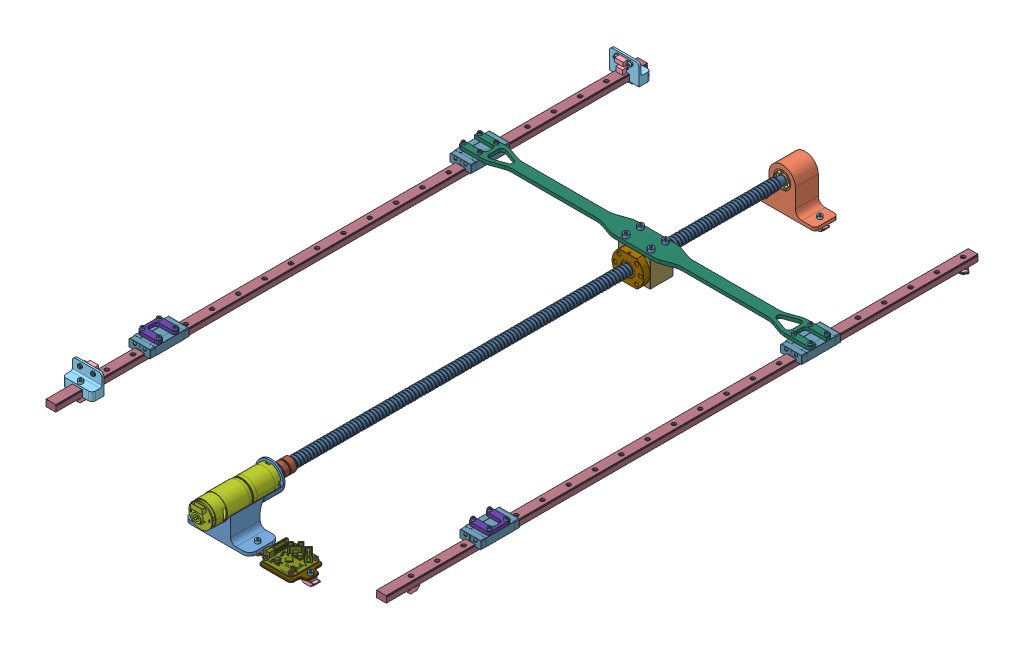
SolidWorks assembly Montaje_Eje_Z_Unity, configuration Predeterminado. Lengths in mm.
Overall size (541.5 84.7 933.8).
85 component instances, 23 part files, 191 mates.
Components (placement in the parent):
- socket head cap screw_iso2-2: socket head cap screw_iso2 [ISO 4762 M3 x 8 - 8N] at (-240.4498 15.8322 -56.4995) x (0 -1 0) z (0 0 1) size (11 5.5 5.5)
- socket head cap screw_iso2-3: socket head cap screw_iso2 [ISO 4762 M3 x 8 - 8N] at (-215.4498 15.8322 -31.4995) x (0 -1 0) z (0 0 1) size (11 5.5 5.5)
- socket head cap screw_iso2-4: socket head cap screw_iso2 [ISO 4762 M3 x 8 - 8N] at (-240.4498 15.8322 -31.4995) x (0 -1 0) z (0 0 1) size (11 5.5 5.5)
- socket head cap screw_iso2-5: socket head cap screw_iso2 [ISO 4762 M3 x 8 - 8N] at (-215.4498 15.8322 -56.4995) x (0 -1 0) z (0.194661 0 0.98087) size (11 5.5 5.5)
- socket head cap screw_iso2-6: socket head cap screw_iso2 [ISO 4762 M3 x 8 - 8N] at (287.5502 15.8322 -56.4995) x (0 -1 0) z (0.194661 0 0.98087) size (11 5.5 5.5)
- socket head cap screw_iso2-7: socket head cap screw_iso2 [ISO 4762 M3 x 8 - 8N] at (262.5502 15.8322 -31.4995) x (0 -1 0) z (0 0 1) size (11 5.5 5.5)
- socket head cap screw_iso2-8: socket head cap screw_iso2 [ISO 4762 M3 x 8 - 8N] at (287.5502 15.8322 -31.4995) x (0 -1 0) z (-0.140271 0 0.990113) size (11 5.5 5.5)
- socket head cap screw_iso2-9: socket head cap screw_iso2 [ISO 4762 M3 x 8 - 8N] at (262.5502 15.8322 -56.4995) x (0 -1 0) z (-0.070011 0 0.997546) size (11 5.5 5.5)
- socket head cap screw_iso2-10: socket head cap screw_iso2 [ISO 4762 M5 x 16 - 16N] at (43.5502 17.8322 -54.9995) x (0 -1 0) z (0 0 1) size (21 8.5 8.5)
- socket head cap screw_iso2-11: socket head cap screw_iso2 [ISO 4762 M5 x 16 - 16N] at (43.5502 17.8322 -32.9995) x (0 -1 0) z (0.965322 0 -0.261062) size (21 8.5 8.5)
- socket head cap screw_iso2-12: socket head cap screw_iso2 [ISO 4762 M5 x 16 - 16N] at (5.5502 17.8322 -32.9995) x (0 -1 0) z (0 0 1) size (21 8.5 8.5)
- socket head cap screw_iso2-13: socket head cap screw_iso2 [ISO 4762 M5 x 16 - 16N] at (5.5502 17.8322 -54.9995) x (0 -1 0) z (0 0 1) size (21 8.5 8.5)
- socket head cap screw_iso2-23: socket head cap screw_iso2 [ISO 4762 M3 x 8 - 8N] at (287.5502 15.8322 456.5005) x (0 -1 0) z (0 0 1) size (11 5.5 5.5)
- socket head cap screw_iso2-24: socket head cap screw_iso2 [ISO 4762 M3 x 8 - 8N] at (287.5502 15.8322 431.5005) x (0 -1 0) z (0 0 1) size (11 5.5 5.5)
- socket head cap screw_iso2-25: socket head cap screw_iso2 [ISO 4762 M3 x 8 - 8N] at (262.5502 15.8322 456.5005) x (0 -1 0) z (0 0 1) size (11 5.5 5.5)
- socket head cap screw_iso2-26: socket head cap screw_iso2 [ISO 4762 M3 x 8 - 8N] at (262.5502 15.8322 431.5005) x (0 -1 0) z (0 0 1) size (11 5.5 5.5)
- socket head cap screw_iso2-27: socket head cap screw_iso2 [ISO 4762 M3 x 8 - 8N] at (-240.4501 15.8323 456.5005) x (0 -1 0) z (0 0 1) size (11 5.5 5.5)
- socket head cap screw_iso2-28: socket head cap screw_iso2 [ISO 4762 M3 x 8 - 8N] at (-215.4501 15.8323 456.5005) x (0 -1 0) z (0 0 1) size (11 5.5 5.5)
- socket head cap screw_iso2-29: socket head cap screw_iso2 [ISO 4762 M3 x 8 - 8N] at (-240.4501 15.8323 431.5005) x (0 -1 0) z (0 0 1) size (11 5.5 5.5)
- socket head cap screw_iso2-30: socket head cap screw_iso2 [ISO 4762 M3 x 8 - 8N] at (-215.4501 15.8323 431.5005) x (0 -1 0) z (0 0 1) size (11 5.5 5.5)
- socket head cap screw_iso2-31: socket head cap screw_iso2 [ISO 4762 M4 x 8 - 8N] at (144.6751 -48.9678 586.0585) x (0 -1 0) z (0 0 1) size (12 7 7)
- socket head cap screw_iso2-33: socket head cap screw_iso2 [ISO 4762 M4 x 8 - 8N] at (84.6751 -48.9678 586.0585) x (0 -1 0) z (0 0 1) size (12 7 7)
- hexa csunk flathd screw_iso2-1: hexa csunk flathd screw_iso2 [ISO 14581 M3x12x12-N] at (133.4451 -55.9678 604.7785) x (-0.795034 0 0.606565) z (0 -1 0) size (5.5 5.5 12)
- hexa csunk flathd screw_iso2-2: hexa csunk flathd screw_iso2 [ISO 14581 M3x12x12-N] at (96.0351 -55.9678 604.7785) x (-0.795034 0 0.606565) z (0 -1 0) size (5.5 5.5 12)
- hexa csunk flathd screw_iso2-4: hexa csunk flathd screw_iso2 [ISO 14581 M3x12x12-N] at (133.4451 -55.9678 567.3685) x (-0.795034 0 0.606565) z (0 -1 0) size (5.5 5.5 12)
- hexa csunk flathd screw_iso2-5: hexa csunk flathd screw_iso2 [ISO 14581 M3x12x12-N] at (96.0351 -55.9678 567.3685) x (-0.795034 0 0.606565) z (0 -1 0) size (5.5 5.5 12)
- hex thin nut chamfered gradeab_iso-1: hex thin nut chamfered gradeab_iso [ISO - 4035 - M3 - N] at (96.0351 -46.1293 604.7785) x (0.635839 0 0.771821) z (0 1 0) size (5.5 6.35 1.8)
- hex thin nut chamfered gradeab_iso-2: hex thin nut chamfered gradeab_iso [ISO - 4035 - M3 - N] at (133.4739 -46.1293 604.6517) x (1 0 0) z (0 1 0) size (5.5 6.35 1.8)
- hex thin nut chamfered gradeab_iso-3: hex thin nut chamfered gradeab_iso [ISO - 4035 - M3 - N] at (133.4739 -46.1293 567.2883) x (1 0 0) z (0 1 0) size (5.5 6.35 1.8)
- hex thin nut chamfered gradeab_iso-4: hex thin nut chamfered gradeab_iso [ISO - 4035 - M3 - N] at (96.0597 -46.1293 567.2629) x (1 0 0) z (0 1 0) size (5.5 6.35 1.8)
- bosch_3842530281_56mh0c106byol9t07uu6uwj7k-1: bosch_3842530281_56mh0c106byol9t07uu6uwj7k [Default] at (84.6751 -58.9678 586.0585) x (1 0 0) z (0 0 1) size (19.6 8.7 10)
- bosch_3842530281_56mh0c106byol9t07uu6uwj7k-2: bosch_3842530281_56mh0c106byol9t07uu6uwj7k [Default] at (144.6751 -58.9678 586.0585) x (1 0 0) z (0 0 1) size (19.6 8.7 10)
- bosch_3842530281_56mh0c106byol9t07uu6uwj7k-3: bosch_3842530281_56mh0c106byol9t07uu6uwj7k [Default] at (64.0502 -58.9678 586.0585) x (1 0 0) z (0 0 1) size (19.6 8.7 10)
- bosch_3842530281_56mh0c106byol9t07uu6uwj7k-4: bosch_3842530281_56mh0c106byol9t07uu6uwj7k [Default] at (-14.9498 -58.9678 586.0585) x (1 0 0) z (0 0 1) size (19.6 8.7 10)
- socket head cap screw_iso-1: socket head cap screw_iso [ISO 4762 M4 x 8 - 8N] at (64.0502 -46.9678 586.0585) x (0 -1 0) z (0 0 1) size (12 7 7)
- socket head cap screw_iso-2: socket head cap screw_iso [ISO 4762 M4 x 8 - 8N] at (-14.9498 -46.9678 586.0585) x (0 -1 0) z (0 0 1) size (12 7 7)
- bosch_3842530281_56mh0c106byol9t07uu6uwj7k-5: bosch_3842530281_56mh0c106byol9t07uu6uwj7k [Default] at (64.5502 -58.9678 -268.9416) x (1 0 0) z (0 0 1) size (19.6 8.7 10)
- bosch_3842530281_56mh0c106byol9t07uu6uwj7k-6: bosch_3842530281_56mh0c106byol9t07uu6uwj7k [Default] at (-15.4498 -58.9678 -268.9416) x (1 0 0) z (0 0 1) size (19.6 8.7 10)
- socket head cap screw_iso-3: socket head cap screw_iso [ISO 4762 M4 x 8 - 8N] at (64.5502 -46.9678 -268.9416) x (0 -1 0) z (0 0 1) size (12 7 7)
- socket head cap screw_iso-4: socket head cap screw_iso [ISO 4762 M4 x 8 - 8N] at (-15.4498 -46.9678 -268.9416) x (0 -1 0) z (0 0 1) size (12 7 7)
- bosch_3842530281_56mh0c106byol9t07uu6uwj7k-7: bosch_3842530281_56mh0c106byol9t07uu6uwj7k [Default] at (-227.9501 -13.9677 -276.5915) x (0 0 1) z (-1 0 0) size (19.6 8.7 10)
- bosch_3842530281_56mh0c106byol9t07uu6uwj7k-8: bosch_3842530281_56mh0c106byol9t07uu6uwj7k [Default] at (-227.9501 -13.9677 563.4085) x (0 0 1) z (-1 0 0) size (19.6 8.7 10)
- bosch_3842530281_56mh0c106byol9t07uu6uwj7k-9: bosch_3842530281_56mh0c106byol9t07uu6uwj7k [Default] at (275.0502 -13.9677 563.7084) x (0 0 -1) z (1 0 0) size (19.6 8.7 10)
- bosch_3842530281_56mh0c106byol9t07uu6uwj7k-10: bosch_3842530281_56mh0c106byol9t07uu6uwj7k [Default] at (275.0502 -13.9677 -276.2916) x (0.798528 0 0.601957) z (-0.601957 0 0.798528) size (19.6 8.7 10)
- socket head cap screw_iso-5: socket head cap screw_iso [ISO 4762 M4 x 16 - 16N] at (-227.9501 6.0323 -276.5915) x (0 -1 0) z (0 0 1) size (20 7 7)
- socket head cap screw_iso-8: socket head cap screw_iso [ISO 4762 M3 x 8 - 8N] at (-237.9501 14.0323 -258.9915) x (0 0 -1) z (1 0 0) size (11 5.5 5.5)
- socket head cap screw_iso-9: socket head cap screw_iso [ISO 4762 M3 x 8 - 8N] at (-217.9501 14.0323 -258.9915) x (0 0 -1) z (1 0 0) size (11 5.5 5.5)
- socket head cap screw_iso-10: socket head cap screw_iso [ISO 4762 M3 x 8 - 8N] at (-217.9501 14.0323 545.8085) x (0 0 1) z (0.923728 0.383049 0) size (11 5.5 5.5)
- socket head cap screw_iso-11: socket head cap screw_iso [ISO 4762 M3 x 8 - 8N] at (-237.9501 14.0323 545.8085) x (0 0 1) z (0.923728 0.383049 0) size (11 5.5 5.5)
- socket head cap screw_iso-12: socket head cap screw_iso [ISO 4762 M4 x 16 - 16N] at (-227.9501 6.0323 563.4085) x (0 -1 0) z (0 0 1) size (20 7 7)
- hex thin nut gradeb_iso-1: hex thin nut gradeb_iso [ISO - 4036 - M3 - N] at (-237.9501 14.0323 555.2085) x (1 0 0) z (0 0 1) size (5.5 6.35 1.8)
- hex thin nut gradeb_iso-2: hex thin nut gradeb_iso [ISO - 4036 - M3 - N] at (-217.9501 14.0323 555.2085) x (1 0 0) z (0 0 1) size (5.5 6.35 1.8)
- hex thin nut gradeb_iso-3: hex thin nut gradeb_iso [ISO - 4036 - M3 - N] at (-237.9501 14.0323 -268.3915) x (-1 -0.000019 0) z (0 0 -1) size (5.5 6.35 1.8)
- hex thin nut gradeb_iso-4: hex thin nut gradeb_iso [ISO - 4036 - M3 - N] at (-217.9501 14.0323 -268.3915) x (-1 -0.000027 0) z (0 0 -1) size (5.5 6.35 1.8)
- Motor_Tornillos-1: Motor_Tornillos [Predeterminado] at (24.5502 -12.1678 506.5645) x (-1 0 0) z (0 0 -1) size (37.2 37.03 132.01)
  - Motor_Tornillos.CATProduct-1: Motor_Tornillos.CATProduct [Predeterminado] at origin size (37.2 37.03 132.01)
    - CHP-36GP-555.CATPart-1: CHP-36GP-555.CATPart [Predeterminado] at (0 0 -31.394) size (37.2 37.03 132.01)
    - ISO_4762_M3x12_STEEL_HEXAGON_SOCKET_HEAD_CAP_SCREW.CATPart-1: ISO_4762_M3x12_STEEL_HEXAGON_SOCKET_HEAD_CAP_SCREW.CATPart [Predeterminado] at (-9.8995 -9.8995 -17.394) x (0 0 1) z (1 0 0) size (15 5.5 5.5)
    - Gathered ISO 4762 SCREW M3x12 STEEL HEXAGON SOCKET HEAD CAP on CircPattern.7.CATProduct-1: Gathered ISO 4762 SCREW M3x12 STEEL HEXAGON SOCKET HEAD CAP on CircPattern.7.CATProduct [Predeterminado] at origin size (25.3 25.3 15)
      - ISO_4762_M3x12_STEEL_HEXAGON_SOCKET_HEAD_CAP_SCREW.CATPart-1: ISO_4762_M3x12_STEEL_HEXAGON_SOCKET_HEAD_CAP_SCREW.CATPart [Predeterminado] at (9.8995 9.8995 -17.394) x (0 0 1) z (-1 0 0) size (15 5.5 5.5)
      - ISO_4762_M3x12_STEEL_HEXAGON_SOCKET_HEAD_CAP_SCREW.CATPart-2: ISO_4762_M3x12_STEEL_HEXAGON_SOCKET_HEAD_CAP_SCREW.CATPart [Predeterminado] at (-9.8995 9.8995 -17.394) x (0 0 1) z (0 -1 0) size (15 5.5 5.5)
      - ISO_4762_M3x12_STEEL_HEXAGON_SOCKET_HEAD_CAP_SCREW.CATPart-3: ISO_4762_M3x12_STEEL_HEXAGON_SOCKET_HEAD_CAP_SCREW.CATPart [Predeterminado] at (9.8995 -9.8995 -17.394) x (0 0 1) z (0 1 0) size (15 5.5 5.5)
- SFU1605-1: SFU1605 [По умолчанию] at (24.5502 -12.1678 -66.4995) x (0 1 0) z (0 0 1) size (40 48 50)
- SCR1605-Z-1: SCR1605-Z [850mm] at (24.5502 -12.1678 -292.8415) x (-0.848768 0.528765 0) z (-0.528765 -0.848768 0) size (16.45 800 18.52)
- Flexible_Coupling_8x8.CATPart-1: Flexible_Coupling_8x8.CATPart [Predeterminado] at (24.5502 -12.1678 545.4741) x (0.984327 -0.176353 0) z (-0.176353 -0.984327 0) size (20 30.8 20)
- HD16-1: HD16 [Default] at (24.5502 7.8322 -26.4995) x (-1 0 0) z (0 0 -1) size (48 40 35)
- MGN15 rail-2: MGN15 rail [MGN15] at (275.0502 -5.9678 -291.2916) x (1 0 0) z (0 0 1) size (15 10 900)
- MGN15C-1: MGN15C [MGN15C] at (275.0502 1.8322 444.0005) x (1 0 0) z (0 0 1) size (32 12 61.91)
- MGN15 rail-3: MGN15 rail [MGN15] at (-227.9501 -5.9677 -291.5915) x (1 0 0) z (0 0 1) size (15 10 900)
- MGN15C-2: MGN15C [MGN15C] at (275.0502 1.8322 -43.9995) x (1 0 0) z (0 0 1) size (32 12 61.91)
- MGN15C-3: MGN15C [MGN15C] at (-227.9501 1.8323 -43.9995) x (1 0 0) z (0 0 1) size (32 12 61.91)
- MGN15C-4: MGN15C [MGN15C] at (-227.9501 1.8323 444.0005) x (1 0 0) z (0 0 1) size (32 12 61.91)
- Viga_Union-1: Viga_Union [Predeterminado] at (23.5502 7.8322 -43.9995) x (1 0 0) z (0 0 1) size (535 5 35)
- PCB_Control_Motores_V2.catpart-1: PCB_Control_Motores_V2.catpart [Predeterminado] at (30.5531 -47.9293 524.0575) x (0 0 1) z (0 1 0) size (48 50.39 14.79)
- Sujección-1: Sujección [Predeterminado] at (275.0502 7.8322 444.0005) x (1 0 0) z (0 0 1) size (31.99 5 35)
- Sujección-2: Sujección [Predeterminado] at (-227.9501 7.8323 444.0005) x (-1 0 0) z (0 0 -1) size (31.99 5 35)
- Soporte_PCB_Motor_Z-1: Soporte_PCB_Motor_Z [Predeterminado] at (114.6751 -55.9678 585.7153) x (1 0 0) z (0 0 1) size (70 3 50)
- Soporte_Motor_Eje_Z-1: Soporte_Motor_Eje_Z [Predeterminado] at (24.5502 -53.4678 563.5585) x (1 0 0) z (0 0 1) size (100 65.01 82.6)
- Soporte_Husillo_Eje_Z-1: Soporte_Husillo_Eje_Z [Predeterminado] at (24.5502 -53.4678 -286.4416) x (1 0 0) z (0 0 1) size (100 63.8 35)
- 6000-Bearing-1: 6000-Bearing [Default] at (24.5502 -12.1678 -259.4416) x (1 0 0) z (0 0 1) size (26 26 8)
- 6000-Bearing-2: 6000-Bearing [Default] at (24.5502 -12.1678 -286.4416) x (1 0 0) z (0 0 1) size (26 26 8)
- End_Stop-1: End_Stop [Predeterminado] at (-227.9501 14.0323 550.4085) x (-1 0 0) z (0 0 -1) size (27 18 10.1)
- End_Stop-2: End_Stop [Predeterminado] at (-227.9501 14.0323 -263.5915) x (1 0 0) z (0 0 1) size (27 18 10.1)
- Soporte_FdC_Eje_Z-1: Soporte_FdC_Eje_Z [Predeterminado] at (-205.4501 0.5323 -272.5915) x (-1 0 0) z (0 0 -1) size (45 31 18)
- Soporte_FdC_Eje_Z-2: Soporte_FdC_Eje_Z [Predeterminado] at (-250.4501 0.5323 559.4085) x (1 0 0) z (0 0 1) size (45 31 18)
Mates (geometry in assembly coordinates):
- Concéntrica2: concentric aligned: circle of Montaje_Pata_Robot.CATProduct-2/Pata_Ext.CATPart-2; circle of Montaje_Pata_Robot.CATProduct-3/Pata_Ext.CATPart-2
- Concéntrica3: concentric aligned: circle of Montaje_Pata_Robot-1/Montaje_Pata_Robot.CATProduct-1/Pata_Ext.CATPart-1; circle of Montaje_Pata_Robot.CATProduct-1/Pata_Ext.CATPart-1
- Distancia1: distance = 473 mm anti-aligned: plane of Montaje_Pata_Robot.CATProduct-2/Pata_Ext.CATPart-2 through (23.6979 293.1537 436.5005) normal (0 0 -1); plane of Montaje_Pata_Robot.CATProduct-3/Pata_Ext.CATPart-1 through (23.6979 293.1537 -36.4995) normal (0 0 1)
- Distancia2: distance = 473 mm anti-aligned: plane of Montaje_Pata_Robot-1/Montaje_Pata_Robot.CATProduct-1/Pata_Ext.CATPart-1 through (23.6979 293.1537 436.5005) normal (0 0 -1); plane of Montaje_Pata_Robot.CATProduct-1/Pata_Ext.CATPart-2 through (23.6979 293.1537 -36.4995) normal (0 0 1)
- Coincidente7: coincident aligned: plane of Montaje_Pata_Robot.CATProduct-1/Pata_Ext.CATPart-1 through (23.6979 293.1537 -51.4995) normal (0 0 -1); plane of Montaje_Pata_Robot.CATProduct-3/Pata_Ext.CATPart-2 through (23.6979 293.1537 -51.4995) normal (0 0 -1)
- Coincidente17: coincident anti-aligned: plane of Motor_Tornillos-1/Motor_Tornillos.CATProduct-1/CHP-36GP-555.CATPart-1 through (24.5502 -12.1678 526.9585) normal (0 0 -1); plane of Flexible_Coupling_8x8.CATPart-1 through (24.5502 -12.1678 526.9585) normal (0 0 1)
- Concéntrica5: concentric aligned: circle of SCR1605-Z-1; circle of Flexible_Coupling_8x8.CATPart-1
- Coincidente18: coincident anti-aligned: plane of SCR1605-Z-1 through (31.3403 -16.398 496.1585) normal (0 0 1); plane of Flexible_Coupling_8x8.CATPart-1 through (24.5502 -12.1678 496.1585) normal (0 0 -1)
- Concéntrica6: concentric aligned: circle of SFU1605-1; circle of SCR1605-Z-1
- Coincidente21: coincident anti-aligned: plane of SFU1605-1 through (24.5502 -12.1678 -26.4995) normal (0 0 -1); plane of HD16-1 through (24.5502 -12.1678 -26.4995) normal (0 0 1)
- Concéntrica8: concentric anti-aligned: circle of SFU1605-1; circle of HD16-1
- Concéntrica9: concentric aligned: circle of SFU1605-1; circle of HD16-1
- Coincidente25: coincident anti-aligned: plane of Montaje_Mesa.CATProduct-1/Montaje_Carril.CATProduct-1/P45L_N10_B_900.CATPart-1 through (281.1501 -10.9677 -291.2916) normal (0 1 0); plane of MGN15 rail-2 through (267.7502 -10.9678 608.7084) normal (0 -1 0)
- Distancia8: distance = 15 mm aligned: plane of MGN15 rail-2 through (282.5502 -10.7678 608.7084) normal (1 0 0); plane of Montaje_Mesa.CATProduct-1/Montaje_Carril.CATProduct-1/P45L_N10_B_900.CATPart-1 through (297.5502 -39.5678 -291.2916) normal (1 0 0)
- Coincidente27: coincident anti-aligned: plane of Montaje_Mesa.CATProduct-1/Montaje_Carril.CATProduct-1/Tapa 45x45.CATPart-1 through (275.05 -33.4678 -291.2916) normal (0 0 1); plane of MGN15 rail-2 through (267.4502 -2.4678 -291.2916) normal (0 0 -1)
- Distancia10: distance = 15 mm aligned: plane of MGN15 rail-3 through (-235.4501 -10.7677 608.4085) normal (-1 0 0); plane of Montaje_Mesa.CATProduct-1/Montaje_Carril.CATProduct-2/P45L_N10_B_900.CATPart-1 through (-250.4501 -39.5678 608.4085) normal (-1 0 0)
- Coincidente32: coincident anti-aligned: plane of MGN15 rail-2 through (282.5502 -10.7678 608.7084) normal (1 0 0); plane of MGN15C-1 through (282.5502 1.8322 465.7005) normal (-1 0 0)
- Coincidente33: coincident anti-aligned: plane of MGN15 rail-2 through (267.7502 -0.9678 608.7084) normal (0 1 0); plane of MGN15C-1 through (275.0502 -0.9678 465.7005) normal (0 -1 0)
- Coincidente34: coincident anti-aligned: plane of MGN15 rail-2 through (267.7502 -0.9678 608.7084) normal (0 1 0); plane of MGN15C-2 through (275.0502 -0.9678 -22.2995) normal (0 -1 0)
- Coincidente35: coincident anti-aligned: plane of MGN15 rail-2 through (282.5502 -10.7678 608.7084) normal (1 0 0); plane of MGN15C-2 through (282.5502 1.8322 -72.4995) normal (-1 0 0)
- Distancia11: distance = 429.2 mm anti-aligned: plane of MGN15C-2 through (275.0502 1.8322 -14.5995) normal (0 0 1); plane of MGN15C-1 through (275.0502 1.8322 414.6005) normal (0 0 -1)
- Coincidente38: coincident anti-aligned: plane of MGN15 rail-3 through (-235.2501 -0.9677 608.4085) normal (0 1 0); plane of MGN15C-4 through (-227.9501 -0.9677 465.7005) normal (0 -1 0)
- Coincidente39: coincident anti-aligned: plane of MGN15 rail-3 through (-220.4501 -10.7677 608.4085) normal (1 0 0); plane of MGN15C-4 through (-220.4501 1.8323 415.5005) normal (-1 0 0)
- Coincidente40: coincident anti-aligned: plane of MGN15 rail-3 through (-235.2501 -0.9677 608.4085) normal (0 1 0); plane of MGN15C-3 through (-227.9501 -0.9677 -22.2995) normal (0 -1 0)
- Coincidente41: coincident anti-aligned: plane of MGN15 rail-3 through (-220.4501 -10.7677 608.4085) normal (1 0 0); plane of MGN15C-3 through (-220.4501 1.8323 -15.4995) normal (-1 0 0)
- Distancia12: distance = 429.2 mm anti-aligned: plane of MGN15C-3 through (-227.9501 1.8323 -14.5995) normal (0 0 1); plane of MGN15C-4 through (-227.9501 1.8323 414.6005) normal (0 0 -1)
- Coincidente44: coincident aligned: plane of MGN15C-2 through (275.0502 1.8322 -73.3995) normal (0 0 -1); plane of MGN15C-3 through (-227.9501 1.8323 -73.3995) normal (0 0 -1)
- Coincidente45: coincident aligned: plane of HD16-1 through (0.5502 7.8322 -61.4995) normal (0 1 0); plane of MGN15C-2 through (275.0502 7.8322 -22.2995) normal (0 1 0)
- Distancia13: distance = 21.9 mm aligned: plane of Montaje_Pata_Robot.CATProduct-1/Pata_Ext.CATPart-1 through (23.6979 293.1537 -51.4995) normal (0 0 -1); plane of MGN15C-2 through (275.0502 1.8322 -73.3995) normal (0 0 -1)
- Coincidente48: coincident anti-aligned: plane of HD16-1 through (0.5502 7.8322 -61.4995) normal (0 1 0); plane of Viga_Union-1 through (23.5502 7.8322 -43.9995) normal (0 -1 0)
- Concéntrica10: concentric anti-aligned: circle of MGN15C-2; circle of Viga_Union-1
- Concéntrica11: concentric anti-aligned: circle of HD16-1; circle of Viga_Union-1
- Paralelo3: parallel aligned: plane of MGN15C-3 through (-227.9501 1.8323 -73.3995) normal (0 0 -1); plane of Viga_Union-1 through (-243.9498 12.8322 -61.4995) normal (0 0 -1)
- Concéntrica13: concentric aligned: circle of Montaje_Pata_Robot-1/Montaje_Pata_Robot.CATProduct-1/Pata_Ext.CATPart-2; circle of Montaje_Pata_Robot.CATProduct-1/Pata_Ext.CATPart-2
- Concéntrica14: concentric aligned: circle of Montaje_Pata_Robot.CATProduct-2/Pata_Ext.CATPart-1; circle of Montaje_Pata_Robot.CATProduct-3/Pata_Ext.CATPart-1
- Concéntrica15: concentric anti-aligned: circle of Montaje_Pata_Robot-1/Montaje_Pata_Robot.CATProduct-1/Pata_Ext.CATPart-2; circle of Montaje_Pata_Robot.CATProduct-2/Pata_Ext.CATPart-1
- Concéntrica16: concentric aligned: circle of Montaje_Pata_Robot.CATProduct-2/Tuerca_Tornillo.CATProduct-6/ISO_4762_M4x20_STEEL_HEXAGON_SOCKET_HEAD_CAP_SCREW.CATPart-1; circle of Montaje_Pata_Robot.CATProduct-3/Tuerca_Tornillo.CATProduct-6/ISO_4762_M4x20_STEEL_HEXAGON_SOCKET_HEAD_CAP_SCREW.CATPart-1
- Concéntrica17: concentric aligned: circle of Montaje_Pata_Robot-1/Montaje_Pata_Robot.CATProduct-1/Pata_Ext.CATPart-2; circle of Montaje_Pata_Robot.CATProduct-1/Pata_Ext.CATPart-2
- Tangente3: tangent anti-aligned: cylinder of Montaje_Pata_Robot.CATProduct-1/Pata_Inter.CATPart-2 through (275.3457 17.6322 -43.9995) axis (0 0 1) radius 10; plane of MGN15C-2 through (275.0502 7.6322 -22.2995) normal (0 1 0)
- Tangente4: tangent anti-aligned: cylinder of Montaje_Pata_Robot.CATProduct-3/Pata_Inter.CATPart-2 through (-227.9501 17.6323 -43.9995) axis (0 0 -1) radius 10; plane of MGN15C-3 through (-227.9501 7.6323 -22.2995) normal (0 1 0)
- Concéntrica18: concentric aligned: circle of Viga_Union-1; circle of socket head cap screw_iso-3
- Coincidente60: coincident anti-aligned: plane of Viga_Union-1 through (23.5502 12.8322 -43.9995) normal (0 1 0); plane of socket head cap screw_iso2-3 through (-212.6998 12.8322 -31.4995) normal (0 -1 0)
- Concéntrica19: concentric aligned: circle of Viga_Union-1; circle of socket head cap screw_iso-4
- Coincidente61: coincident anti-aligned: plane of Viga_Union-1 through (23.5502 12.8322 -43.9995) normal (0 1 0); plane of socket head cap screw_iso2-4 through (-237.6998 12.8322 -31.4995) normal (0 -1 0)
- Concéntrica20: concentric anti-aligned: circle of Viga_Union-1; circle of socket head cap screw_iso-2
- Concéntrica21: concentric aligned: circle of Viga_Union-1; circle of socket head cap screw_iso-5
- Coincidente62: coincident anti-aligned: plane of Viga_Union-1 through (23.5502 12.8322 -43.9995) normal (0 1 0); plane of socket head cap screw_iso2-5 through (-212.7524 12.8322 -57.0348) normal (0 -1 0)
- Coincidente63: coincident anti-aligned: plane of Viga_Union-1 through (23.5502 12.8322 -43.9995) normal (0 1 0); plane of socket head cap screw_iso2-2 through (-237.6998 12.8322 -56.4995) normal (0 -1 0)
- Concéntrica22: concentric aligned: circle of Viga_Union-1; circle of socket head cap screw_iso-7
- Coincidente64: coincident anti-aligned: plane of Viga_Union-1 through (23.5502 12.8322 -43.9995) normal (0 1 0); plane of socket head cap screw_iso2-7 through (265.3002 12.8322 -31.4995) normal (0 -1 0)
- Concéntrica23: concentric aligned: circle of Viga_Union-1; circle of socket head cap screw_iso-8
- Coincidente65: coincident anti-aligned: plane of Viga_Union-1 through (23.5502 12.8322 -43.9995) normal (0 1 0); plane of socket head cap screw_iso2-8 through (290.273 12.8322 -31.1138) normal (0 -1 0)
- Concéntrica24: concentric aligned: circle of Viga_Union-1; circle of socket head cap screw_iso-9
- Coincidente66: coincident anti-aligned: plane of Viga_Union-1 through (23.5502 12.8322 -43.9995) normal (0 1 0); plane of socket head cap screw_iso2-9 through (265.2934 12.8322 -56.307) normal (0 -1 0)
- Coincidente67: coincident anti-aligned: plane of Viga_Union-1 through (23.5502 12.8322 -43.9995) normal (0 1 0); plane of socket head cap screw_iso2-6 through (290.2476 12.8322 -57.0348) normal (0 -1 0)
- Concéntrica25: concentric aligned: circle of Viga_Union-1; circle of socket head cap screw_iso-6
- Concéntrica27: concentric aligned: circle of HD16-1; circle of Viga_Union-1
- Concéntrica28: concentric aligned: cylinder of Viga_Union-1 through (43.5502 7.8322 -54.9995) axis (0 1 0) radius 2.55; cylinder of socket head cap screw_iso2-10 through (43.5502 49.5822 -54.9995) axis (0 1 0) radius 4.25
- Coincidente68: coincident anti-aligned: plane of Viga_Union-1 through (23.5502 12.8322 -43.9995) normal (0 1 0); plane of socket head cap screw_iso2-10 through (47.8002 12.8322 -54.9995) normal (0 -1 0)
- Concéntrica29: concentric aligned: cylinder of Viga_Union-1 through (43.5502 7.8322 -32.9995) axis (0 1 0) radius 2.55; cylinder of socket head cap screw_iso2-11 through (43.5502 49.5822 -32.9995) axis (0 1 0) radius 4.25
- Coincidente69: coincident anti-aligned: plane of Viga_Union-1 through (23.5502 12.8322 -43.9995) normal (0 1 0); plane of socket head cap screw_iso2-11 through (42.4407 12.8322 -37.1021) normal (0 -1 0)
- Concéntrica30: concentric aligned: cylinder of Viga_Union-1 through (5.5502 7.8322 -32.9995) axis (0 1 0) radius 2.55; cylinder of socket head cap screw_iso2-12 through (5.5502 49.5822 -32.9995) axis (0 1 0) radius 4.25
- Coincidente70: coincident anti-aligned: plane of Viga_Union-1 through (23.5502 12.8322 -43.9995) normal (0 1 0); plane of socket head cap screw_iso2-12 through (9.8002 12.8322 -32.9995) normal (0 -1 0)
- Concéntrica31: concentric aligned: cylinder of Viga_Union-1 through (5.5502 7.8322 -54.9995) axis (0 1 0) radius 2.55; cylinder of socket head cap screw_iso2-13 through (5.5502 49.5822 -54.9995) axis (0 1 0) radius 4.25
- Coincidente71: coincident anti-aligned: plane of Viga_Union-1 through (23.5502 12.8322 -43.9995) normal (0 1 0); plane of socket head cap screw_iso2-13 through (9.8002 12.8322 -54.9995) normal (0 -1 0)
- Coincidente78: coincident anti-aligned: line of Montaje_Mesa.CATProduct-1/P45L_N10_B_550.CATPart-1 through (-251.45 -58.9678 608.5586) axis (1 0 0); line of Armario-1/Caja-1 through (94.55 -58.9678 608.5586) axis (-1 0 0)
- Coincidente80: coincident aligned: line of Montaje_Mesa.CATProduct-1/P45L_N10_B_550.CATPart-1 through (-251.45 -58.9678 608.5586) axis (0 -1 0); line of Armario-1/Caja-1 through (-251.45 -68.9678 608.5586) axis (0 -1 0)
- Distancia14: distance = 22.5 mm: point of Montaje_Pata_Robot.CATProduct-3/Tuerca_Tornillo.CATProduct-4/1587_M4_Tuerca_Ciega.CATPart-1; plane of Montaje_Mesa.CATProduct-1/Montaje_Carril.CATProduct-2/P45L_N10_B_900.CATPart-1 through (-250.4501 -39.5678 608.4085) normal (-1 0 0)
- Distancia15: distance = 483.5249 mm: point of Montaje_Pata_Robot.CATProduct-1/Pata_Ext.CATPart-2; point of Montaje_Pata_Robot.CATProduct-3/Pata_Ext.CATPart-1
- Concéntrica32: concentric aligned: cylinder of MGN15C-1 through (287.5502 7.8322 456.5005) axis (0 1 0) radius 1.25; circle of Sujección-1
- Coincidente84: coincident anti-aligned: plane of MGN15C-1 through (275.0502 7.8322 465.7005) normal (0 1 0); plane of Sujección-1 through (275.0502 7.8322 444.0005) normal (0 -1 0)
- Concéntrica33: concentric anti-aligned: circle of MGN15C-1; circle of Sujección-1
- Concéntrica34: concentric aligned: circle of MGN15C-4; circle of Sujección-2
- Coincidente85: coincident anti-aligned: plane of MGN15C-4 through (-227.9501 7.8323 465.7005) normal (0 1 0); plane of Sujección-2 through (-227.9501 7.8323 444.0005) normal (0 -1 0)
- Concéntrica35: concentric aligned: circle of MGN15C-4; circle of Sujección-2
- Concéntrica44: concentric anti-aligned: cylinder of Sujección-1 through (287.5502 12.8322 456.5005) axis (0 -1 0) radius 1.55; cylinder of socket head cap screw_iso2-23 through (287.5502 47.5822 456.5005) axis (0 1 0) radius 2.75
- Coincidente94: coincident anti-aligned: plane of Sujección-1 through (275.0502 12.8322 444.0005) normal (0 1 0); plane of socket head cap screw_iso2-23 through (290.3002 12.8322 456.5005) normal (0 -1 0)
- Concéntrica45: concentric anti-aligned: cylinder of Sujección-1 through (287.5502 12.8322 431.5005) axis (0 -1 0) radius 1.55; cylinder of socket head cap screw_iso2-24 through (287.5502 47.5822 431.5005) axis (0 1 0) radius 2.75
- Coincidente95: coincident anti-aligned: plane of Sujección-1 through (275.0502 12.8322 444.0005) normal (0 1 0); plane of socket head cap screw_iso2-24 through (290.3002 12.8322 431.5005) normal (0 -1 0)
- Concéntrica46: concentric anti-aligned: cylinder of Sujección-1 through (262.5502 12.8322 456.5005) axis (0 -1 0) radius 1.55; cylinder of socket head cap screw_iso2-25 through (262.5502 47.5822 456.5005) axis (0 1 0) radius 2.75
- Coincidente96: coincident anti-aligned: plane of Sujección-1 through (275.0502 12.8322 444.0005) normal (0 1 0); plane of socket head cap screw_iso2-25 through (265.3002 12.8322 456.5005) normal (0 -1 0)
- Concéntrica47: concentric anti-aligned: cylinder of Sujección-1 through (262.5502 12.8322 431.5005) axis (0 -1 0) radius 1.55; cylinder of socket head cap screw_iso2-26 through (262.5502 47.5822 431.5005) axis (0 1 0) radius 2.75
- Coincidente97: coincident anti-aligned: plane of Sujección-1 through (275.0502 12.8322 444.0005) normal (0 1 0); plane of socket head cap screw_iso2-26 through (265.3002 12.8322 431.5005) normal (0 -1 0)
- Concéntrica48: concentric anti-aligned: cylinder of Sujección-2 through (-240.4501 12.8323 456.5005) axis (0 -1 0) radius 1.55; cylinder of socket head cap screw_iso2-27 through (-240.4501 47.5823 456.5005) axis (0 1 0) radius 2.75
- Coincidente98: coincident anti-aligned: plane of Sujección-2 through (-227.9501 12.8323 444.0005) normal (0 1 0); plane of socket head cap screw_iso2-27 through (-237.7001 12.8323 456.5005) normal (0 -1 0)
- Concéntrica49: concentric anti-aligned: cylinder of Sujección-2 through (-215.4501 12.8323 456.5005) axis (0 -1 0) radius 1.55; cylinder of socket head cap screw_iso2-28 through (-215.4501 47.5823 456.5005) axis (0 1 0) radius 2.75
- Coincidente99: coincident anti-aligned: plane of Sujección-2 through (-227.9501 12.8323 444.0005) normal (0 1 0); plane of socket head cap screw_iso2-28 through (-212.7001 12.8323 456.5005) normal (0 -1 0)
- Concéntrica50: concentric anti-aligned: cylinder of Sujección-2 through (-240.4501 12.8323 431.5005) axis (0 -1 0) radius 1.55; cylinder of socket head cap screw_iso2-29 through (-240.4501 47.5823 431.5005) axis (0 1 0) radius 2.75
- Coincidente100: coincident anti-aligned: plane of Sujección-2 through (-227.9501 12.8323 444.0005) normal (0 1 0); plane of socket head cap screw_iso2-29 through (-237.7001 12.8323 431.5005) normal (0 -1 0)
- Concéntrica51: concentric anti-aligned: cylinder of Sujección-2 through (-215.4501 12.8323 431.5005) axis (0 -1 0) radius 1.55; cylinder of socket head cap screw_iso2-30 through (-215.4501 47.5823 431.5005) axis (0 1 0) radius 2.75
- Coincidente101: coincident anti-aligned: plane of Sujección-2 through (-227.9501 12.8323 444.0005) normal (0 1 0); plane of socket head cap screw_iso2-30 through (-212.7001 12.8323 431.5005) normal (0 -1 0)
- Coincidente102: coincident anti-aligned: plane of Montaje_Mesa.CATProduct-1/P45L_N10_B_550.CATPart-1 through (-251.45 -55.9678 579.9585) normal (0 1 0); plane of Soporte_PCB_Motor_Z-1 through (114.6751 -55.9678 585.7153) normal (0 -1 0)
- Distancia18: distance = 1 mm aligned: plane of PCB_Control_Motores_V2.catpart-1 through (138.6751 -49.5208 568.0555) normal (1 0 0); plane of Soporte_PCB_Motor_Z-1 through (139.6751 -52.9678 611.0585) normal (1 0 0)
- Coincidente116: coincident anti-aligned: plane of Montaje_Mesa.CATProduct-1/P45L_N10_B_550.CATPart-1 through (-251.45 -57.7679 591.0585) normal (0 0 -1); plane of bosch_3842530281_56mh0c106byol9t07uu6uwj7k-1 through (84.6751 -61.9328 591.0585) normal (0 0 1)
- Coincidente117: coincident aligned: plane of Montaje_Mesa.CATProduct-1/P45L_N10_B_550.CATPart-1 through (-251.45 -55.9678 579.9585) normal (0 1 0); plane of bosch_3842530281_56mh0c106byol9t07uu6uwj7k-1 through (84.6751 -55.9678 586.0585) normal (0 1 0)
- Coincidente118: coincident aligned: plane of Montaje_Mesa.CATProduct-1/P45L_N10_B_550.CATPart-1 through (-251.45 -55.9678 579.9585) normal (0 1 0); plane of bosch_3842530281_56mh0c106byol9t07uu6uwj7k-2 through (144.6751 -55.9678 586.0585) normal (0 1 0)
- Coincidente119: coincident anti-aligned: plane of Montaje_Mesa.CATProduct-1/P45L_N10_B_550.CATPart-1 through (-251.45 -57.7679 591.0585) normal (0 0 -1); plane of bosch_3842530281_56mh0c106byol9t07uu6uwj7k-2 through (144.6751 -61.9328 591.0585) normal (0 0 1)
- Concéntrica63: concentric anti-aligned: circle of Soporte_PCB_Motor_Z-1; circle of bosch_3842530281_56mh0c106byol9t07uu6uwj7k-2
- Concéntrica64: concentric anti-aligned: circle of Soporte_PCB_Motor_Z-1; circle of bosch_3842530281_56mh0c106byol9t07uu6uwj7k-1
- Concéntrica65: concentric anti-aligned: cylinder of Soporte_PCB_Motor_Z-1 through (144.6751 -52.9678 586.0585) axis (0 -1 0) radius 2.05; cylinder of socket head cap screw_iso-31 through (144.6751 -17.2178 586.0585) axis (0 1 0) radius 3.5
- Coincidente121: coincident anti-aligned: plane of Soporte_PCB_Motor_Z-1 through (114.6751 -52.9678 585.7153) normal (0 1 0); plane of socket head cap screw_iso-31 through (148.1751 -52.9678 586.0585) normal (0 -1 0)
- Concéntrica66: concentric aligned: cylinder of bosch_3842530281_56mh0c106byol9t07uu6uwj7k-1 through (84.6751 -60.3178 586.0585) axis (0 1 0) radius 1.65; cylinder of socket head cap screw_iso-33 through (84.6751 -17.2178 586.0585) axis (0 1 0) radius 3.5
- Coincidente123: coincident anti-aligned: plane of Soporte_PCB_Motor_Z-1 through (114.6751 -52.9678 585.7153) normal (0 1 0); plane of socket head cap screw_iso-33 through (88.1751 -52.9678 586.0585) normal (0 -1 0)
- Concéntrica69: concentric aligned: circle of Soporte_PCB_Motor_Z-1; circle of hexa csunk flathd screw_iso-1
- Coincidente124: coincident anti-aligned: plane of Montaje_Mesa.CATProduct-1/P45L_N10_B_550.CATPart-1 through (-251.45 -55.9678 579.9585) normal (0 1 0); plane of hexa csunk flathd screw_iso-1 through (133.4451 -55.9678 604.7785) normal (0 -1 0)
- Coincidente125: coincident anti-aligned: plane of Montaje_Mesa.CATProduct-1/P45L_N10_B_550.CATPart-1 through (-251.45 -55.9678 579.9585) normal (0 1 0); plane of hexa csunk flathd screw_iso-4 through (133.4451 -55.9678 567.3685) normal (0 -1 0)
- Concéntrica73: concentric aligned: circle of Soporte_PCB_Motor_Z-1; circle of hexa csunk flathd screw_iso-4
- Coincidente126: coincident anti-aligned: plane of Montaje_Mesa.CATProduct-1/P45L_N10_B_550.CATPart-1 through (-251.45 -55.9678 579.9585) normal (0 1 0); plane of hexa csunk flathd screw_iso-2 through (96.0351 -55.9678 604.7785) normal (0 -1 0)
- Concéntrica74: concentric aligned: circle of Soporte_PCB_Motor_Z-1; circle of hexa csunk flathd screw_iso-2
- Coincidente127: coincident anti-aligned: plane of Montaje_Mesa.CATProduct-1/P45L_N10_B_550.CATPart-1 through (-251.45 -55.9678 579.9585) normal (0 1 0); plane of hexa csunk flathd screw_iso-5 through (96.0351 -55.9678 567.3685) normal (0 -1 0)
- Concéntrica75: concentric anti-aligned: cylinder of Soporte_PCB_Motor_Z-1 through (96.0351 -52.9678 567.3685) axis (0 -1 0) radius 1.55; circle of hexa csunk flathd screw_iso-5
- Concéntrica77: concentric aligned: cone of hexa csunk flathd screw_iso-2 through (96.0351 -44.1298 604.7785) axis (0 1 0); cylinder of hex thin nut chamfered gradeab_iso-1 through (96.0351 -71.1668 604.7785) axis (0 1 0) radius 1.5
- Coincidente129: coincident anti-aligned: plane of PCB_Control_Motores_V2.catpart-1 through (93.4611 -47.9293 564.8455) normal (0 1 0); plane of hex thin nut chamfered gradeab_iso-1 through (98.4859 -47.9293 602.7595) normal (0 -1 0)
- Concéntrica78: concentric aligned: cylinder of PCB_Control_Motores_V2.catpart-1 through (133.4739 -49.5208 604.6517) axis (0 1 0) radius 1.65; cylinder of hex thin nut chamfered gradeab_iso-2 through (133.4739 -71.1668 604.6517) axis (0 1 0) radius 1.5
- Coincidente130: coincident anti-aligned: plane of PCB_Control_Motores_V2.catpart-1 through (93.4611 -47.9293 564.8455) normal (0 1 0); plane of hex thin nut chamfered gradeab_iso-2 through (133.4739 -47.9293 601.4762) normal (0 -1 0)
- Concéntrica79: concentric aligned: cylinder of PCB_Control_Motores_V2.catpart-1 through (133.4739 -49.5208 567.2883) axis (0 1 0) radius 1.65; cylinder of hex thin nut chamfered gradeab_iso-3 through (133.4739 -71.1668 567.2883) axis (0 1 0) radius 1.5
- Coincidente131: coincident anti-aligned: plane of PCB_Control_Motores_V2.catpart-1 through (93.4611 -47.9293 564.8455) normal (0 1 0); plane of hex thin nut chamfered gradeab_iso-3 through (133.4739 -47.9293 564.1128) normal (0 -1 0)
- Concéntrica80: concentric aligned: cylinder of PCB_Control_Motores_V2.catpart-1 through (96.0597 -49.5208 567.2629) axis (0 1 0) radius 1.65; cylinder of hex thin nut chamfered gradeab_iso-4 through (96.0597 -71.1668 567.2629) axis (0 1 0) radius 1.5
- Coincidente132: coincident anti-aligned: plane of PCB_Control_Motores_V2.catpart-1 through (93.4611 -47.9293 564.8455) normal (0 1 0); plane of hex thin nut chamfered gradeab_iso-4 through (96.0597 -47.9293 564.0874) normal (0 -1 0)
- Coincidente134: coincident anti-aligned: plane of Montaje_Mesa.CATProduct-1/P45L_N10_B_550.CATPart-1 through (-251.45 -55.9678 579.9585) normal (0 1 0); plane of Soporte_Motor_Eje_Z-1 through (-25.4498 -55.9678 608.5585) normal (0 -1 0)
- Coincidente135: coincident aligned: plane of Montaje_Mesa.CATProduct-1/P45L_N10_B_550.CATPart-1 through (-251.45 -55.9678 579.9585) normal (0 1 0); plane of bosch_3842530281_56mh0c106byol9t07uu6uwj7k-4 through (-14.9498 -55.9678 586.0585) normal (0 1 0)
- Coincidente136: coincident anti-aligned: plane of Montaje_Mesa.CATProduct-1/P45L_N10_B_550.CATPart-1 through (-251.45 -57.7679 591.0585) normal (0 0 -1); plane of bosch_3842530281_56mh0c106byol9t07uu6uwj7k-4 through (-14.9498 -61.9328 591.0585) normal (0 0 1)
- Coincidente137: coincident anti-aligned: plane of Montaje_Mesa.CATProduct-1/P45L_N10_B_550.CATPart-1 through (-251.45 -57.7679 591.0585) normal (0 0 -1); plane of bosch_3842530281_56mh0c106byol9t07uu6uwj7k-3 through (64.0502 -61.9328 591.0585) normal (0 0 1)
- Coincidente138: coincident aligned: plane of Montaje_Mesa.CATProduct-1/P45L_N10_B_550.CATPart-1 through (-251.45 -55.9678 579.9585) normal (0 1 0); plane of bosch_3842530281_56mh0c106byol9t07uu6uwj7k-3 through (64.0502 -55.9678 586.0585) normal (0 1 0)
- Concéntrica81: concentric anti-aligned: circle of Soporte_Motor_Eje_Z-1; circle of bosch_3842530281_56mh0c106byol9t07uu6uwj7k-4
- Concéntrica82: concentric anti-aligned: circle of Soporte_Motor_Eje_Z-1; circle of bosch_3842530281_56mh0c106byol9t07uu6uwj7k-3
- Concéntrica85: concentric anti-aligned: circle of Motor_Tornillos-1/Motor_Tornillos.CATProduct-1/CHP-36GP-555.CATPart-1; circle of Soporte_Motor_Eje_Z-1
- Paralelo4: parallel: line of Motor_Tornillos-1/Motor_Tornillos.CATProduct-1/CHP-36GP-555.CATPart-1 through (15.7502 3.2472 639.5585) axis (0 -1 0); plane of Montaje_Mesa.CATProduct-1/Montaje_Carril.CATProduct-2/P45L_N10_B_900.CATPart-1 through (-205.45 -27.3677 608.4085) normal (1 0 0)
- Distancia19: distance = 25 mm aligned: plane of Motor_Tornillos-1/Motor_Tornillos.CATProduct-1/CHP-36GP-555.CATPart-1 through (24.5502 -12.1678 633.5585) normal (0 0 1); plane of Soporte_Motor_Eje_Z-1 through (24.5502 -12.1678 608.5585) normal (0 0 1)
- Concéntrica86: concentric aligned: cylinder of Soporte_Motor_Eje_Z-1 through (64.0502 -55.9678 586.0585) axis (0 1 0) radius 2.05; cylinder of socket head cap screw_iso-1 through (64.0502 -15.2178 586.0585) axis (0 1 0) radius 3.5
- Coincidente143: coincident anti-aligned: plane of Soporte_Motor_Eje_Z-1 through (45.5502 -50.9678 608.5585) normal (0 1 0); plane of socket head cap screw_iso-1 through (67.5502 -50.9678 586.0585) normal (0 -1 0)
- Concéntrica87: concentric aligned: cylinder of Soporte_Motor_Eje_Z-1 through (-14.9498 -55.9678 586.0585) axis (0 1 0) radius 2.05; cylinder of socket head cap screw_iso-2 through (-14.9498 -15.2178 586.0585) axis (0 1 0) radius 3.5
- Coincidente144: coincident anti-aligned: plane of Soporte_Motor_Eje_Z-1 through (-25.4498 -50.9678 608.5585) normal (0 1 0); plane of socket head cap screw_iso-2 through (-11.4498 -50.9678 586.0585) normal (0 -1 0)
- Concéntrica96: concentric anti-aligned: circle of Soporte_Motor_Eje_Z-1; circle of Soporte_Husillo_Eje_Z-1
- Coincidente148: coincident anti-aligned: plane of Montaje_Mesa.CATProduct-1/P45L_N10_B_550.CATPart-2 through (-251.45 -55.9678 -275.0416) normal (0 1 0); plane of Soporte_Husillo_Eje_Z-1 through (24.5502 -55.9678 -251.4416) normal (0 -1 0)
- Coincidente153: coincident anti-aligned: plane of Montaje_Mesa.CATProduct-1/P45L_N10_B_550.CATPart-2 through (-251.45 -61.6679 -273.9416) normal (0 0 1); plane of bosch_3842530281_56mh0c106byol9t07uu6uwj7k-6 through (-15.4498 -61.9328 -273.9416) normal (0 0 -1)
- Coincidente154: coincident anti-aligned: plane of Montaje_Mesa.CATProduct-1/P45L_N10_B_550.CATPart-2 through (-251.45 -61.6679 -273.9416) normal (0 0 1); plane of bosch_3842530281_56mh0c106byol9t07uu6uwj7k-5 through (64.5502 -61.9328 -273.9416) normal (0 0 -1)
- Coincidente155: coincident aligned: plane of Montaje_Mesa.CATProduct-1/P45L_N10_B_550.CATPart-2 through (-251.45 -55.9678 -275.0416) normal (0 1 0); plane of bosch_3842530281_56mh0c106byol9t07uu6uwj7k-5 through (64.5502 -55.9678 -268.9416) normal (0 1 0)
- Coincidente156: coincident aligned: plane of Montaje_Mesa.CATProduct-1/P45L_N10_B_550.CATPart-2 through (-251.45 -55.9678 -275.0416) normal (0 1 0); plane of bosch_3842530281_56mh0c106byol9t07uu6uwj7k-6 through (-15.4498 -55.9678 -268.9416) normal (0 1 0)
- Concéntrica97: concentric anti-aligned: circle of Soporte_Husillo_Eje_Z-1; circle of bosch_3842530281_56mh0c106byol9t07uu6uwj7k-5
- Concéntrica98: concentric anti-aligned: circle of Soporte_Husillo_Eje_Z-1; circle of bosch_3842530281_56mh0c106byol9t07uu6uwj7k-6
- Concéntrica99: concentric aligned: cylinder of Soporte_Husillo_Eje_Z-1 through (64.5502 -55.9678 -268.9416) axis (0 1 0) radius 2.05; cylinder of socket head cap screw_iso-3 through (64.5502 -15.2178 -268.9416) axis (0 1 0) radius 3.5
- Coincidente157: coincident anti-aligned: plane of Soporte_Husillo_Eje_Z-1 through (24.5502 -50.9678 -251.4416) normal (0 1 0); plane of socket head cap screw_iso-3 through (68.0502 -50.9678 -268.9416) normal (0 -1 0)
- Concéntrica100: concentric aligned: cylinder of Soporte_Husillo_Eje_Z-1 through (-15.4498 -55.9678 -268.9416) axis (0 1 0) radius 2.05; cylinder of socket head cap screw_iso-4 through (-15.4498 -15.2178 -268.9416) axis (0 1 0) radius 3.5
- Coincidente158: coincident anti-aligned: plane of Soporte_Husillo_Eje_Z-1 through (24.5502 -50.9678 -251.4416) normal (0 1 0); plane of socket head cap screw_iso-4 through (-11.9498 -50.9678 -268.9416) normal (0 -1 0)
- Concéntrica101: concentric anti-aligned: circle of Soporte_Husillo_Eje_Z-1; circle of 6000-Bearing-1
- Coincidente159: coincident aligned: plane of Soporte_Husillo_Eje_Z-1 through (24.5502 -53.4678 -251.4416) normal (0 0 1); plane of 6000-Bearing-1 through (24.5502 -12.1678 -251.4416) normal (0 0 1)
- Coincidente160: coincident aligned: plane of Soporte_Husillo_Eje_Z-1 through (24.5502 -53.4678 -286.4416) normal (0 0 -1); plane of 6000-Bearing-2 through (24.5502 -12.1678 -286.4416) normal (0 0 -1)
- Concéntrica102: concentric anti-aligned: circle of Soporte_Husillo_Eje_Z-1; circle of 6000-Bearing-2
- Coincidente164: coincident anti-aligned: plane of Montaje_Mesa.CATProduct-1/Montaje_Carril.CATProduct-2/P45L_N10_B_900.CATPart-1 through (-222.9501 -12.7678 608.4085) normal (-1 0 0); plane of bosch_3842530281_56mh0c106byol9t07uu6uwj7k-8 through (-222.9501 -16.9327 563.4085) normal (1 0 0)
- Coincidente165: coincident aligned: plane of Montaje_Mesa.CATProduct-1/Montaje_Carril.CATProduct-2/P45L_N10_B_900.CATPart-1 through (-234.0501 -10.9677 608.4085) normal (0 1 0); plane of bosch_3842530281_56mh0c106byol9t07uu6uwj7k-8 through (-227.9501 -10.9677 563.4085) normal (0 1 0)
- Coincidente166: coincident aligned: plane of Montaje_Mesa.CATProduct-1/Montaje_Carril.CATProduct-1/P45L_N10_B_900.CATPart-1 through (281.1501 -10.9677 -291.2916) normal (0 1 0); plane of bosch_3842530281_56mh0c106byol9t07uu6uwj7k-10 through (275.0502 -10.9677 -276.2916) normal (0 1 0)
- Coincidente168: coincident aligned: plane of Montaje_Mesa.CATProduct-1/Montaje_Carril.CATProduct-1/P45L_N10_B_900.CATPart-1 through (281.1501 -10.9677 -291.2916) normal (0 1 0); plane of bosch_3842530281_56mh0c106byol9t07uu6uwj7k-9 through (275.0502 -10.9677 563.7084) normal (0 1 0)
- Concéntrica110: concentric aligned: circle of MGN15 rail-3; circle of bosch_3842530281_56mh0c106byol9t07uu6uwj7k-7
- Concéntrica112: concentric anti-aligned: circle of MGN15 rail-2; circle of bosch_3842530281_56mh0c106byol9t07uu6uwj7k-9
- Concéntrica113: concentric anti-aligned: circle of MGN15 rail-2; circle of bosch_3842530281_56mh0c106byol9t07uu6uwj7k-10
- Coincidente169: coincident anti-aligned: plane of Montaje_Mesa.CATProduct-1/Montaje_Carril.CATProduct-2/P45L_N10_B_900.CATPart-1 through (-234.0501 -10.9677 608.4085) normal (0 1 0); plane of MGN15 rail-3 through (-235.2501 -10.9677 608.4085) normal (0 -1 0)
- Coincidente170: coincident: line of Montaje_Mesa.CATProduct-1/Montaje_Carril.CATProduct-2/P45L_N10_B_900.CATPart-1 through (-247.4501 -10.9677 -291.5915) axis (1 0 0); plane of MGN15 rail-3 through (-235.5501 -2.4677 -291.5915) normal (0 0 -1)
- Concéntrica114: concentric aligned: circle of HD16-1; circle of Soporte_Husillo_Eje_Z-1
- Concéntrica116: concentric anti-aligned: circle of MGN15 rail-3; circle of Soporte_FdC_Eje_Z-1
- Paralelo6: parallel aligned: plane of Montaje_Mesa.CATProduct-1/Montaje_Carril.CATProduct-2/P45L_N10_B_900.CATPart-1 through (-250.4501 -39.5678 608.4085) normal (-1 0 0); plane of Soporte_FdC_Eje_Z-1 through (-250.4501 0.5323 -272.5915) normal (-1 0 0)
- Coincidente178: coincident anti-aligned: plane of Montaje_Mesa.CATProduct-1/Montaje_Carril.CATProduct-2/P45L_N10_B_900.CATPart-1 through (-234.0501 -10.9677 608.4085) normal (0 1 0); plane of Soporte_FdC_Eje_Z-1 through (-205.4501 -10.9677 -272.5915) normal (0 -1 0)
- Coincidente179: coincident anti-aligned: plane of End_Stop-2 through (-227.9501 14.0323 -263.5915) normal (0 0 -1); plane of Soporte_FdC_Eje_Z-1 through (-250.4501 -0.9677 -263.5915) normal (0 0 1)
- Concéntrica122: concentric aligned: circle of End_Stop-2; circle of Soporte_FdC_Eje_Z-1
- Concéntrica123: concentric aligned: circle of End_Stop-2; circle of Soporte_FdC_Eje_Z-1
- Concéntrica124: concentric aligned: cylinder of Soporte_FdC_Eje_Z-1 through (-227.9501 -0.9677 -276.5915) axis (0 1 0) radius 2; cylinder of socket head cap screw_iso-5 through (-227.9501 37.7823 -276.5915) axis (0 1 0) radius 3.5
- Coincidente180: coincident anti-aligned: plane of Soporte_FdC_Eje_Z-1 through (-250.4501 2.0323 -281.5915) normal (0 1 0); plane of socket head cap screw_iso-5 through (-224.4501 2.0323 -276.5915) normal (0 -1 0)
- Concéntrica126: concentric anti-aligned: cylinder of End_Stop-2 through (-237.9501 14.0323 -262.7915) axis (0 0 -1) radius 1.5; cylinder of socket head cap screw_iso-8 through (-237.9501 14.0323 -227.2415) axis (0 0 1) radius 2.75
- Coincidente181: coincident anti-aligned: plane of End_Stop-2 through (-227.9501 14.0323 -261.9915) normal (0 0 1); plane of socket head cap screw_iso-8 through (-237.9501 16.7823 -261.9915) normal (0 0 -1)
- Concéntrica127: concentric anti-aligned: cylinder of End_Stop-2 through (-217.9501 14.0323 -262.7915) axis (0 0 -1) radius 1.5; cylinder of socket head cap screw_iso-9 through (-217.9501 14.0323 -227.2415) axis (0 0 1) radius 2.75
- Coincidente182: coincident anti-aligned: plane of End_Stop-2 through (-227.9501 14.0323 -261.9915) normal (0 0 1); plane of socket head cap screw_iso-9 through (-217.9501 16.7823 -261.9915) normal (0 0 -1)
- Concéntrica128: concentric anti-aligned: cylinder of End_Stop-1 through (-217.9501 14.0323 549.6085) axis (0 0 1) radius 1.5; cylinder of socket head cap screw_iso-10 through (-217.9501 14.0323 514.0585) axis (0 0 -1) radius 2.75
- Coincidente183: coincident anti-aligned: plane of End_Stop-1 through (-227.9501 14.0323 548.8085) normal (0 0 -1); plane of socket head cap screw_iso-10 through (-216.8967 11.4921 548.8085) normal (0 0 1)
- Concéntrica129: concentric anti-aligned: cylinder of End_Stop-1 through (-237.9501 14.0323 549.6085) axis (0 0 1) radius 1.5; cylinder of socket head cap screw_iso-11 through (-237.9501 14.0323 514.0585) axis (0 0 -1) radius 2.75
- Coincidente184: coincident anti-aligned: plane of End_Stop-1 through (-227.9501 14.0323 548.8085) normal (0 0 -1); plane of socket head cap screw_iso-11 through (-236.8967 11.4921 548.8085) normal (0 0 1)
- Concéntrica130: concentric anti-aligned: circle of MGN15 rail-3; circle of Soporte_FdC_Eje_Z-2
- Paralelo7: parallel aligned: plane of Montaje_Mesa.CATProduct-1/Montaje_Carril.CATProduct-2/P45L_N10_B_900.CATPart-1 through (-250.4501 -39.5678 608.4085) normal (-1 0 0); plane of Soporte_FdC_Eje_Z-2 through (-250.4501 0.5323 559.4085) normal (-1 0 0)
- Coincidente186: coincident anti-aligned: plane of Montaje_Mesa.CATProduct-1/Montaje_Carril.CATProduct-2/P45L_N10_B_900.CATPart-1 through (-234.0501 -10.9677 608.4085) normal (0 1 0); plane of Soporte_FdC_Eje_Z-2 through (-250.4501 -10.9677 559.4085) normal (0 -1 0)
- Coincidente187: coincident anti-aligned: plane of End_Stop-1 through (-227.9501 14.0323 550.4085) normal (0 0 1); plane of Soporte_FdC_Eje_Z-2 through (-205.4501 -0.9677 550.4085) normal (0 0 -1)
- Concéntrica131: concentric aligned: circle of socket head cap screw_iso-11; circle of Soporte_FdC_Eje_Z-2
- Concéntrica132: concentric aligned: circle of socket head cap screw_iso-10; circle of Soporte_FdC_Eje_Z-2
- Concéntrica133: concentric aligned: cylinder of Soporte_FdC_Eje_Z-2 through (-227.9501 -0.9677 563.4085) axis (0 1 0) radius 2; cylinder of socket head cap screw_iso-12 through (-227.9501 37.7823 563.4085) axis (0 1 0) radius 3.5
- Coincidente188: coincident anti-aligned: plane of Soporte_FdC_Eje_Z-2 through (-205.4501 2.0323 568.4085) normal (0 1 0); plane of socket head cap screw_iso-12 through (-224.4501 2.0323 563.4085) normal (0 -1 0)
- Concéntrica134: concentric anti-aligned: cylinder of Soporte_FdC_Eje_Z-2 through (-237.9501 14.0323 568.4085) axis (0 0 -1) radius 1.55; cylinder of hex thin nut gradeb_iso-1 through (-237.9501 14.0323 530.171) axis (0 0 1) radius 1.5
- Coincidente189: coincident anti-aligned: plane of Soporte_FdC_Eje_Z-2 through (-205.4501 2.0323 553.4085) normal (0 0 1); plane of hex thin nut gradeb_iso-1 through (-237.9501 17.2078 553.4085) normal (0 0 -1)
- Concéntrica135: concentric anti-aligned: cylinder of Soporte_FdC_Eje_Z-2 through (-217.9501 14.0323 568.4085) axis (0 0 -1) radius 1.55; cylinder of hex thin nut gradeb_iso-2 through (-217.9501 14.0323 530.171) axis (0 0 1) radius 1.5
- Coincidente190: coincident anti-aligned: plane of Soporte_FdC_Eje_Z-2 through (-205.4501 2.0323 553.4085) normal (0 0 1); plane of hex thin nut gradeb_iso-2 through (-217.9501 17.2078 553.4085) normal (0 0 -1)
- Concéntrica136: concentric aligned: cone of socket head cap screw_iso-8 through (-237.9501 14.0323 -269.9915) axis (0 0 -1); cylinder of hex thin nut gradeb_iso-3 through (-237.9501 14.0323 -243.354) axis (0 0 -1) radius 1.5
- Coincidente191: coincident anti-aligned: plane of Soporte_FdC_Eje_Z-1 through (-250.4501 2.0323 -266.5915) normal (0 0 -1); plane of hex thin nut gradeb_iso-3 through (-237.9502 17.2078 -266.5915) normal (0 0 1)
- Concéntrica137: concentric anti-aligned: cylinder of Soporte_FdC_Eje_Z-1 through (-217.9501 14.0323 -281.5915) axis (0 0 1) radius 1.55; cylinder of hex thin nut gradeb_iso-4 through (-217.9501 14.0323 -243.354) axis (0 0 -1) radius 1.5
- Coincidente192: coincident anti-aligned: plane of Soporte_FdC_Eje_Z-1 through (-250.4501 2.0323 -266.5915) normal (0 0 -1); plane of hex thin nut gradeb_iso-4 through (-217.9502 17.2078 -266.5915) normal (0 0 1)
